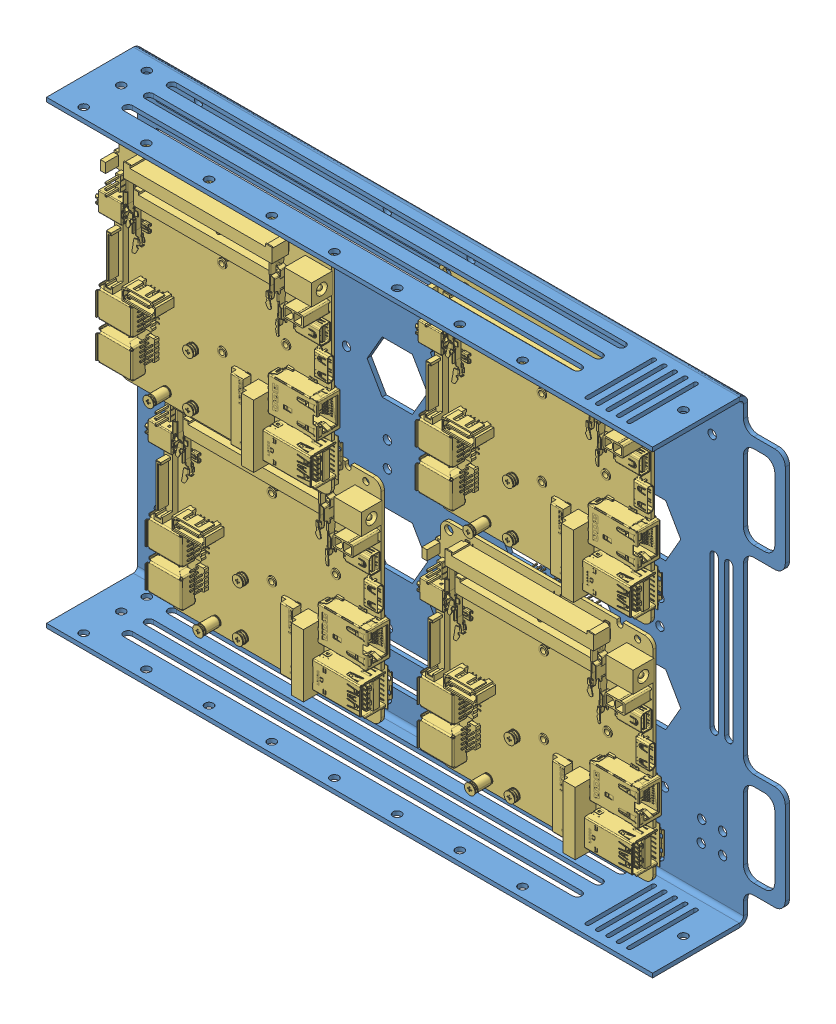
SolidWorks assembly kubebox_tray_nuc, configuration Predeterminado. Lengths in mm.
Overall size (310 220 50.81).
6 component instances, 3 part files, 5 mates.
Components (placement in the parent):
- kubebox_tray-1: kubebox_tray [Predeterminado] at (-106.1016 -89.1854 250) size (310 220 45.5)
- 2-56_Press-Fit_Nut_Sheet_Metal _Min.Thickness_.03-1: 2-56_Press-Fit_Nut_Sheet_Metal _Min.Thickness_.03 [95185A103] at (-166.1016 -74.1854 246.222) x (0.974986 0.222265 0) z (0 0 -1) size (6.35 6.35 2.81)
- D34010WYB-D54250WYB.step-1: D34010WYB-D54250WYB.step [Default] at (30.3984 74.3146 259.8713) x (0 -1 0) z (-1 0 0) size (101.61 21.41 108.83)
- D34010WYB-D54250WYB.step-2: D34010WYB-D54250WYB.step [Default] at (30.3984 -32.6854 259.053) x (0 -1 0) z (-1 0 0) size (101.61 21.41 108.83)
- D34010WYB-D54250WYB.step-3: D34010WYB-D54250WYB.step [Default] at (-100.0016 -32.6854 258.6983) x (0 -1 0) z (-1 0 0) size (101.61 21.41 108.83)
- D34010WYB-D54250WYB.step-4: D34010WYB-D54250WYB.step [Default] at (-100.0016 74.3146 282.4911) x (0 -1 0) z (-1 0 0) size (101.61 21.41 108.83)
Mates (geometry in assembly coordinates):
- Coincident2: coincident anti-aligned: plane of kubebox_tray-1 through (118.8984 -19.1854 248) normal (0 0 -1); plane of 2-56_Press-Fit_Nut_Sheet_Metal _Min.Thickness_.03-1 through (-166.1016 -74.1854 248) normal (0 0 1)
- Concentric4: concentric aligned: cylinder of kubebox_tray-1 through (-146.9016 -80.1854 248) axis (0 0 1) radius 2; cylinder of D34010WYB-D54250WYB.step-3 through (-146.9016 -80.1854 258.6983) axis (0 0 1) radius 2
- Concentric5: concentric aligned: cylinder of kubebox_tray-1 through (-146.9016 26.8146 248) axis (0 0 1) radius 2; cylinder of D34010WYB-D54250WYB.step-4 through (-146.9016 26.8146 282.4911) axis (0 0 1) radius 2
- Concentric6: concentric aligned: cylinder of kubebox_tray-1 through (-16.5016 26.8146 248) axis (0 0 1) radius 2; cylinder of D34010WYB-D54250WYB.step-1 through (-16.5016 26.8146 259.8713) axis (0 0 1) radius 2
- Concentric7: concentric aligned: cylinder of kubebox_tray-1 through (-16.5016 14.8146 248) axis (0 0 1) radius 2; cylinder of D34010WYB-D54250WYB.step-2 through (-16.5016 14.8146 259.053) axis (0 0 1) radius 2
